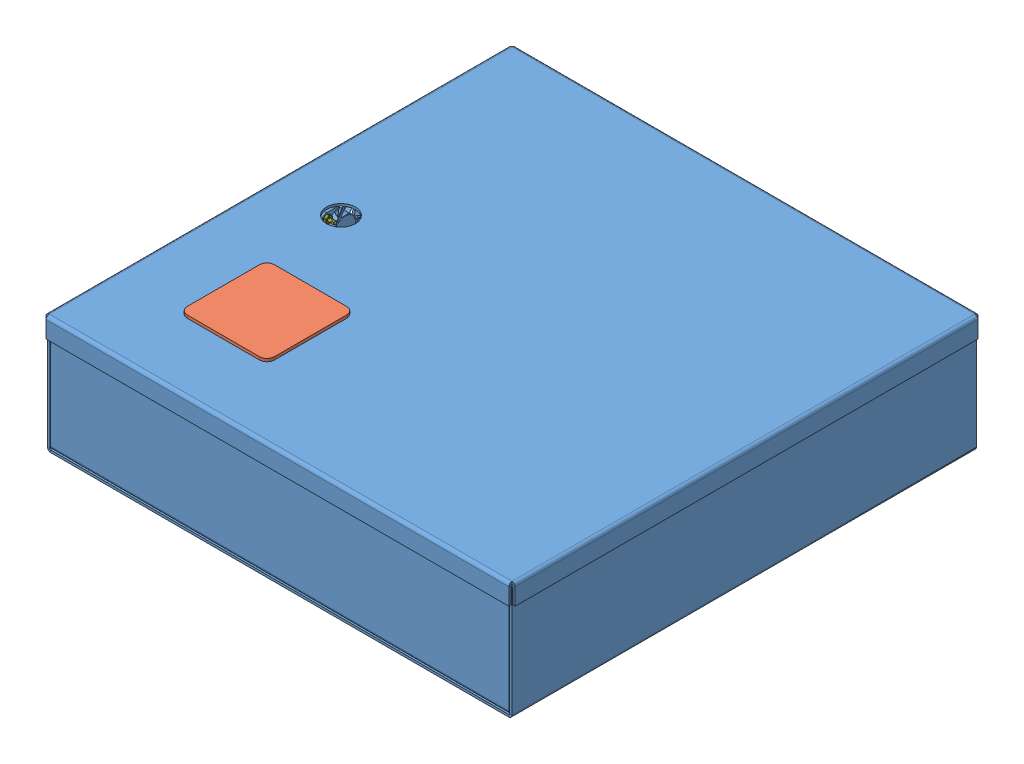
SolidWorks assembly elc box assebly, configuration Default. Lengths in mm.
Overall size (410.46 136 412.7).
107 component instances, 22 part files, 29 mates.
Components (placement in the parent):
- Electrical Enclosure 16 in-1: Electrical Enclosure 16 in [Default] at (-5.7869 193.9093 67.1276) size (410.46 103.63 410.46)
- elc component panel-1: elc component panel [Default] at (423.6423 -1.464 537.2069) x (-1 0 0) z (0 0 -1) size (400.05 136 400.05)
  - elc plate-1: elc plate [Default] at (226.2293 207.4053 266.8793) size (400.05 1.59 400.05)
  - power supply with standoffs-1: power supply with standoffs [Default] at (-1.4024 133.9192 27.3055) size (115.2 58.27 215)
    - __-1: __ [По умолчанию] at (110.1067 83.0736 152.0488) size (115.2 50.11 215)
    - 95783A055_NYLON 6 6 MALE-FEMALE THREADED HEX STANDOFF-1: 95783A055_NYLON 6 6 MALE-FEMALE THREADED HEX STANDOFF [95783A055] at (85.1067 81.4236 77.0488) x (0 1 0) z (0 0 1) size (13.03 5.2 4.5)
    - 95783A055_NYLON 6 6 MALE-FEMALE THREADED HEX STANDOFF-2: 95783A055_NYLON 6 6 MALE-FEMALE THREADED HEX STANDOFF [95783A055] at (135.1067 81.4236 77.0488) x (0 1 0) z (-0.939028 0 -0.343839) size (13.03 5.2 4.5)
    - 95783A055_NYLON 6 6 MALE-FEMALE THREADED HEX STANDOFF-3: 95783A055_NYLON 6 6 MALE-FEMALE THREADED HEX STANDOFF [95783A055] at (135.1067 81.4236 227.0488) x (0 1 0) z (-0.996262 0 -0.086381) size (13.03 5.2 4.5)
    - 95783A055_NYLON 6 6 MALE-FEMALE THREADED HEX STANDOFF-4: 95783A055_NYLON 6 6 MALE-FEMALE THREADED HEX STANDOFF [95783A055] at (85.1067 81.4236 227.0488) x (0 1 0) z (-0.990494 0 -0.137554) size (13.03 5.2 4.5)
  - arduino board assembly-1: arduino board assembly [Default] at (144.0018 173.6976 442.1285) x (0 0 -1) z (1 0 0) size (100 30.86 52.88)
    - ArduinoMega2560 CORRECTED-1: ArduinoMega2560 CORRECTED [Default] at (48.9673 43.2952 72.715) size (100 11.65 51.63)
    - breakout board-1: breakout board [Default] at (48.9673 54.2952 72.715) size (100 7 51.63)
    - 95783A055_NYLON 6 6 MALE-FEMALE THREADED HEX STANDOFF-1: 95783A055_NYLON 6 6 MALE-FEMALE THREADED HEX STANDOFF [95783A055] at (84.2031 36.9452 49.5995) x (0 -1 0) z (0 0 1) size (13.03 5.2 4.5)
    - 95783A055_NYLON 6 6 MALE-FEMALE THREADED HEX STANDOFF-2: 95783A055_NYLON 6 6 MALE-FEMALE THREADED HEX STANDOFF [95783A055] at (3.483 36.9452 49.7272) x (0 -1 0) z (0 0 1) size (13.03 5.2 4.5)
    - 95783A055_NYLON 6 6 MALE-FEMALE THREADED HEX STANDOFF-3: 95783A055_NYLON 6 6 MALE-FEMALE THREADED HEX STANDOFF [95783A055] at (9.6911 36.9452 96.9805) x (0 -1 0) z (0 0 1) size (13.03 5.2 4.5)
    - 91290A110_BLACK-OXIDE CLASS 12.9 SOCKET HEAD CAP SCREW-1: 91290A110_BLACK-OXIDE CLASS 12.9 SOCKET HEAD CAP SCREW [91290A110] at (9.6911 39.2952 96.9805) x (1 0 0) z (0 -1 0) size (5.5 5.5 8.18)
    - 91290A110_BLACK-OXIDE CLASS 12.9 SOCKET HEAD CAP SCREW-2: 91290A110_BLACK-OXIDE CLASS 12.9 SOCKET HEAD CAP SCREW [91290A110] at (84.2031 39.2952 49.5995) x (1 0 0) z (0 -1 0) size (5.5 5.5 8.18)
    - 91290A110_BLACK-OXIDE CLASS 12.9 SOCKET HEAD CAP SCREW-3: 91290A110_BLACK-OXIDE CLASS 12.9 SOCKET HEAD CAP SCREW [91290A110] at (3.483 39.2952 49.7272) x (1 0 0) z (0 -1 0) size (5.5 5.5 8.18)
  - din rail assmbly-1: din rail assmbly [Default] at (168.8197 101.8607 336.151) x (0 0 -1) z (1 0 0) size (90.31 80.69 125)
    - DIN 59_0-1: DIN 59_0 [00] at (103.6081 107.1321 54.2926) size (35 7.5 125)
    - 3812830-1: 3812830 [Default] at (104.4524 140.3713 142.3959) x (0 0 1) z (-1 0 0) size (6.2 76.69 90.31)
      - 3812830A-1: 3812830A [Default] at (-75.9936 -29.2392 18.3443) size (6.2 76.69 90.31)
      - 3812830B-1: 3812830B [Default] at (-75.3936 25.9608 19.6) size (5 19.3 28)
    - 3812830-2: 3812830 [Default] at (104.4524 140.3713 148.5959) x (0 0 1) z (-1 0 0) size (6.2 76.69 90.31)
      - 3812830A-1: 3812830A [Default] at (-75.9936 -29.2392 18.3443) size (6.2 76.69 90.31)
      - 3812830B-1: 3812830B [Default] at (-75.3936 25.9608 19.6) size (5 19.3 28)
    - 3812830-3: 3812830 [Default] at (104.4524 140.3713 154.7959) x (0 0 1) z (-1 0 0) size (6.2 76.69 90.31)
      - 3812830A-1: 3812830A [Default] at (-75.9936 -29.2392 18.3443) size (6.2 76.69 90.31)
      - 3812830B-1: 3812830B [Default] at (-75.3936 25.9608 19.6) size (5 19.3 28)
    - 3812830-4: 3812830 [Default] at (104.4524 140.3713 160.9959) x (0 0 1) z (-1 0 0) size (6.2 76.69 90.31)
      - 3812830A-1: 3812830A [Default] at (-75.9936 -29.2392 18.3443) size (6.2 76.69 90.31)
      - 3812830B-1: 3812830B [Default] at (-75.3936 25.9608 19.6) size (5 19.3 28)
    - SEIMENS 8WA1 808 DIN RAIL END RETAINER-1: SEIMENS 8WA1 808 DIN RAIL END RETAINER [Default] at (102.6081 107.6321 61.4023) size (45 44.95 10)
    - dinrail_Terminal-1: dinrail_Terminal [Default] at (121.1081 114.6321 91.2023) size (48 46.85 5.15)
    - dinrail_Terminal-2: dinrail_Terminal [Default] at (121.1081 114.6321 96.3523) size (48 46.85 5.15)
    - dinrail_Terminal-3: dinrail_Terminal [Default] at (121.1081 114.6321 101.5023) size (48 46.85 5.15)
    - dinrail_Terminal-4: dinrail_Terminal [Default] at (121.1081 114.6321 106.6523) size (48 46.85 5.15)
    - dinrail_Terminal-5: dinrail_Terminal [Default] at (121.1081 114.6321 111.8023) size (48 46.85 5.15)
    - 3812830-5: 3812830 [Default] at (104.4524 140.3713 205.3459) x (0 0 1) z (-1 0 0) size (6.2 76.69 90.31)
      - 3812830A-1: 3812830A [Default] at (-75.9936 -29.2392 18.3443) size (6.2 76.69 90.31)
      - 3812830B-1: 3812830B [Default] at (-75.3936 25.9608 19.6) size (5 19.3 28)
    - 3812830-6: 3812830 [Default] at (104.4524 140.3713 199.1459) x (0 0 1) z (-1 0 0) size (6.2 76.69 90.31)
      - 3812830A-1: 3812830A [Default] at (-75.9936 -29.2392 18.3443) size (6.2 76.69 90.31)
      - 3812830B-1: 3812830B [Default] at (-75.3936 25.9608 19.6) size (5 19.3 28)
    - 3812830-7: 3812830 [Default] at (104.4524 140.3713 192.9459) x (0 0 1) z (-1 0 0) size (6.2 76.69 90.31)
      - 3812830A-1: 3812830A [Default] at (-75.9936 -29.2392 18.3443) size (6.2 76.69 90.31)
      - 3812830B-1: 3812830B [Default] at (-75.3936 25.9608 19.6) size (5 19.3 28)
    - dinrail_Terminal-6: dinrail_Terminal [Default] at (121.1081 114.6321 135.5523) size (48 46.85 5.15)
    - dinrail_Terminal-7: dinrail_Terminal [Default] at (121.1081 114.6321 140.7023) size (48 46.85 5.15)
    - dinrail_Terminal-8: dinrail_Terminal [Default] at (121.1081 114.6321 145.8523) size (48 46.85 5.15)
    - dinrail_Terminal-9: dinrail_Terminal [Default] at (121.1081 114.6321 151.0023) size (48 46.85 5.15)
    - dinrail_Terminal-10: dinrail_Terminal [Default] at (121.1081 114.6321 156.1523) size (48 46.85 5.15)
    - SEIMENS 8WA1 808 DIN RAIL END RETAINER-3: SEIMENS 8WA1 808 DIN RAIL END RETAINER [Default] at (102.6081 107.6321 166.3023) size (45 44.95 10)
  - arduino board assembly-2: arduino board assembly [Default] at (46.0623 173.6976 442.1285) x (0 0 -1) z (1 0 0) size (100 30.86 52.88)
    - ArduinoMega2560 CORRECTED-1: ArduinoMega2560 CORRECTED [Default] at (48.9673 43.2952 72.715) size (100 11.65 51.63)
    - breakout board-1: breakout board [Default] at (48.9673 54.2952 72.715) size (100 7 51.63)
    - 95783A055_NYLON 6 6 MALE-FEMALE THREADED HEX STANDOFF-1: 95783A055_NYLON 6 6 MALE-FEMALE THREADED HEX STANDOFF [95783A055] at (84.2031 36.9452 49.5995) x (0 -1 0) z (0 0 1) size (13.03 5.2 4.5)
    - 95783A055_NYLON 6 6 MALE-FEMALE THREADED HEX STANDOFF-2: 95783A055_NYLON 6 6 MALE-FEMALE THREADED HEX STANDOFF [95783A055] at (3.483 36.9452 49.7272) x (0 -1 0) z (0 0 1) size (13.03 5.2 4.5)
    - 95783A055_NYLON 6 6 MALE-FEMALE THREADED HEX STANDOFF-3: 95783A055_NYLON 6 6 MALE-FEMALE THREADED HEX STANDOFF [95783A055] at (9.6911 36.9452 96.9805) x (0 -1 0) z (0 0 1) size (13.03 5.2 4.5)
    - 91290A110_BLACK-OXIDE CLASS 12.9 SOCKET HEAD CAP SCREW-1: 91290A110_BLACK-OXIDE CLASS 12.9 SOCKET HEAD CAP SCREW [91290A110] at (9.6911 39.2952 96.9805) x (1 0 0) z (0 -1 0) size (5.5 5.5 8.18)
    - 91290A110_BLACK-OXIDE CLASS 12.9 SOCKET HEAD CAP SCREW-2: 91290A110_BLACK-OXIDE CLASS 12.9 SOCKET HEAD CAP SCREW [91290A110] at (84.2031 39.2952 49.5995) x (1 0 0) z (0 -1 0) size (5.5 5.5 8.18)
    - 91290A110_BLACK-OXIDE CLASS 12.9 SOCKET HEAD CAP SCREW-3: 91290A110_BLACK-OXIDE CLASS 12.9 SOCKET HEAD CAP SCREW [91290A110] at (3.483 39.2952 49.7272) x (1 0 0) z (0 -1 0) size (5.5 5.5 8.18)
  - small panduit 1-1: small panduit 1 [Default] at (435.7793 210.2628 310.0077) size (368.3 30.38 16.31)
  - small panduit 2-1: small panduit 2 [Default] at (196.2827 210.2628 -91.8457) x (0 0 -1) z (1 0 0) size (133.35 30.38 16.31)
  - small panduit 3-1: small panduit 3 [Default] at (581.8293 210.2628 160.3509) size (222.25 30.38 16.31)
  - small panduit 2-2: small panduit 2 [Default] at (70.2327 210.2628 57.8111) x (0 0 -1) z (1 0 0) size (133.35 30.38 16.31)
  - small panduit 2-3: small panduit 2 [Default] at (168.1721 210.2628 57.8111) x (0 0 -1) z (1 0 0) size (133.35 30.38 16.31)
  - small panduit 2-4: small panduit 2 [Default] at (266.1116 210.2628 57.8111) x (0 0 -1) z (1 0 0) size (133.35 30.38 16.31)
  - small panduit 2-5: small panduit 2 [Default] at (667.965 210.2628 443.3577) size (133.35 30.38 16.31)
  - 92497A200_ZINC YELLOW-CHROMATE PLATED STEEL HEX NUT-1: 92497A200_ZINC YELLOW-CHROMATE PLATED STEEL HEX NUT [92497A200] at (95.7896 206.2053 438.6455) x (1 0 0) z (0 1 0) size (5.5 6.35 2.78)
  - 92497A200_ZINC YELLOW-CHROMATE PLATED STEEL HEX NUT-2: 92497A200_ZINC YELLOW-CHROMATE PLATED STEEL HEX NUT [92497A200] at (95.6618 206.2053 357.9254) x (1 0 0) z (0 1 0) size (5.5 6.35 2.78)
  - 92497A200_ZINC YELLOW-CHROMATE PLATED STEEL HEX NUT-3: 92497A200_ZINC YELLOW-CHROMATE PLATED STEEL HEX NUT [92497A200] at (143.0428 206.2053 432.4374) x (1 0 0) z (0 1 0) size (5.5 6.35 2.78)
  - 92497A200_ZINC YELLOW-CHROMATE PLATED STEEL HEX NUT-4: 92497A200_ZINC YELLOW-CHROMATE PLATED STEEL HEX NUT [92497A200] at (193.729 206.2053 438.6455) x (1 0 0) z (0 1 0) size (5.5 6.35 2.78)
  - 92497A200_ZINC YELLOW-CHROMATE PLATED STEEL HEX NUT-5: 92497A200_ZINC YELLOW-CHROMATE PLATED STEEL HEX NUT [92497A200] at (193.6013 206.2053 357.9254) x (1 0 0) z (0 1 0) size (5.5 6.35 2.78)
  - 92497A200_ZINC YELLOW-CHROMATE PLATED STEEL HEX NUT-6: 92497A200_ZINC YELLOW-CHROMATE PLATED STEEL HEX NUT [92497A200] at (240.9823 206.2053 432.4374) x (1 0 0) z (0 1 0) size (5.5 6.35 2.78)
  - 92095A177_18-8 SS BUTTON-HEAD SOCKET CAP SCREW-1: 92095A177_18-8 SS BUTTON-HEAD SOCKET CAP SCREW [92095A177] at (133.7043 205.7553 254.3543) x (1 0 0) z (0 -1 0) size (5.7 5.7 6.94)
  - 92095A177_18-8 SS BUTTON-HEAD SOCKET CAP SCREW-2: 92095A177_18-8 SS BUTTON-HEAD SOCKET CAP SCREW [92095A177] at (83.7043 205.7553 254.3543) x (1 0 0) z (0 -1 0) size (5.7 5.7 6.94)
  - 92095A177_18-8 SS BUTTON-HEAD SOCKET CAP SCREW-3: 92095A177_18-8 SS BUTTON-HEAD SOCKET CAP SCREW [92095A177] at (133.7043 205.7553 104.3543) x (1 0 0) z (0 -1 0) size (5.7 5.7 6.94)
  - 92095A177_18-8 SS BUTTON-HEAD SOCKET CAP SCREW-4: 92095A177_18-8 SS BUTTON-HEAD SOCKET CAP SCREW [92095A177] at (83.7043 205.7553 104.3543) x (1 0 0) z (0 -1 0) size (5.7 5.7 6.94)
  - 94060A146_PAN HEAD DRILLING SCREW FOR METAL-1: 94060A146_PAN HEAD DRILLING SCREW FOR METAL [94060A146] at (70.2327 204.3097 431.8261) x (1 0 0) z (0 1 0) size (6.86 6.86 33.5)
  - 94060A146_PAN HEAD DRILLING SCREW FOR METAL-2: 94060A146_PAN HEAD DRILLING SCREW FOR METAL [94060A146] at (70.2327 204.3097 327.6861) x (1 0 0) z (0 1 0) size (6.86 6.86 33.5)
  - 94060A146_PAN HEAD DRILLING SCREW FOR METAL-3: 94060A146_PAN HEAD DRILLING SCREW FOR METAL [94060A146] at (168.1721 204.3097 327.6861) x (1 0 0) z (0 1 0) size (6.86 6.86 33.5)
  - 94060A146_PAN HEAD DRILLING SCREW FOR METAL-4: 94060A146_PAN HEAD DRILLING SCREW FOR METAL [94060A146] at (168.1721 204.3097 431.8261) x (1 0 0) z (0 1 0) size (6.86 6.86 33.5)
  - 94060A146_PAN HEAD DRILLING SCREW FOR METAL-5: 94060A146_PAN HEAD DRILLING SCREW FOR METAL [94060A146] at (266.1116 204.3097 431.8261) x (1 0 0) z (0 1 0) size (6.86 6.86 33.5)
  - 94060A146_PAN HEAD DRILLING SCREW FOR METAL-6: 94060A146_PAN HEAD DRILLING SCREW FOR METAL [94060A146] at (266.1116 204.3097 327.6861) x (1 0 0) z (0 1 0) size (6.86 6.86 33.5)
  - 94060A146_PAN HEAD DRILLING SCREW FOR METAL-7: 94060A146_PAN HEAD DRILLING SCREW FOR METAL [94060A146] at (293.95 204.3097 443.3577) x (1 0 0) z (0 1 0) size (6.86 6.86 33.5)
  - 94060A146_PAN HEAD DRILLING SCREW FOR METAL-8: 94060A146_PAN HEAD DRILLING SCREW FOR METAL [94060A146] at (398.09 204.3097 443.3577) x (1 0 0) z (0 1 0) size (6.86 6.86 33.5)
  - 94060A146_PAN HEAD DRILLING SCREW FOR METAL-9: 94060A146_PAN HEAD DRILLING SCREW FOR METAL [94060A146] at (386.2493 204.3097 160.3509) x (1 0 0) z (0 1 0) size (6.86 6.86 33.5)
  - 94060A146_PAN HEAD DRILLING SCREW FOR METAL-10: 94060A146_PAN HEAD DRILLING SCREW FOR METAL [94060A146] at (196.2827 204.3097 178.0293) x (1 0 0) z (0 1 0) size (6.86 6.86 33.5)
  - 94060A146_PAN HEAD DRILLING SCREW FOR METAL-11: 94060A146_PAN HEAD DRILLING SCREW FOR METAL [94060A146] at (196.2827 204.3097 282.1693) x (1 0 0) z (0 1 0) size (6.86 6.86 33.5)
  - 94060A146_PAN HEAD DRILLING SCREW FOR METAL-12: 94060A146_PAN HEAD DRILLING SCREW FOR METAL [94060A146] at (207.8143 204.3097 160.3509) x (1 0 0) z (0 1 0) size (6.86 6.86 33.5)
  - 94060A146_PAN HEAD DRILLING SCREW FOR METAL-13: 94060A146_PAN HEAD DRILLING SCREW FOR METAL [94060A146] at (388.7893 204.3097 310.0077) x (1 0 0) z (0 1 0) size (6.86 6.86 33.5)
  - 94060A146_PAN HEAD DRILLING SCREW FOR METAL-14: 94060A146_PAN HEAD DRILLING SCREW FOR METAL [94060A146] at (61.7643 204.3097 310.0077) x (1 0 0) z (0 1 0) size (6.86 6.86 33.5)
  - 94060A146_PAN HEAD DRILLING SCREW FOR METAL-15: 94060A146_PAN HEAD DRILLING SCREW FOR METAL [94060A146] at (233.1123 204.0397 232.5429) x (1 0 0) z (0 1 0) size (6.86 6.86 33.5)
  - 94060A146_PAN HEAD DRILLING SCREW FOR METAL-16: 94060A146_PAN HEAD DRILLING SCREW FOR METAL [94060A146] at (341.1123 204.0397 232.5429) x (1 0 0) z (0 1 0) size (6.86 6.86 33.5)
- 40x40x10 DC Fan-1: 40x40x10 DC Fan [Default] at (249.8006 244.7093 74.4096) size (49.86 40.69 10.5)
- 40x40x10 DC Fan-2: 40x40x10 DC Fan [Default] at (1.4951 244.7093 225.8776) x (0 0 -1) z (1 0 0) size (49.86 40.69 10.5)
- fan hole cover-1: fan hole cover [Default] at (90.1997 300.0813 377.5156) x (-1 0 0) z (0 0 1) size (76.2 12.7 76.2)
- 92095A185_18-8 SS BUTTON-HEAD SOCKET CAP SCREW-1: 92095A185_18-8 SS BUTTON-HEAD SOCKET CAP SCREW [92095A185] at (265.8026 260.7113 65.4776) x (-0.923728 -0.383049 0) z (0 0 -1) size (5.7 5.7 22.02)
- 92095A185_18-8 SS BUTTON-HEAD SOCKET CAP SCREW-2: 92095A185_18-8 SS BUTTON-HEAD SOCKET CAP SCREW [92095A185] at (233.7986 228.7073 65.4776) x (-0.923728 -0.383049 0) z (0 0 -1) size (5.7 5.7 22.02)
- 92095A185_18-8 SS BUTTON-HEAD SOCKET CAP SCREW-3: 92095A185_18-8 SS BUTTON-HEAD SOCKET CAP SCREW [92095A185] at (-7.4369 260.7113 241.8796) x (0 0 1) z (-1 0 0) size (5.7 5.7 22.02)
- 92095A185_18-8 SS BUTTON-HEAD SOCKET CAP SCREW-4: 92095A185_18-8 SS BUTTON-HEAD SOCKET CAP SCREW [92095A185] at (-7.4369 228.7073 209.8756) x (0 0 1) z (-1 0 0) size (5.7 5.7 22.02)
- 92497A200_ZINC YELLOW-CHROMATE PLATED STEEL HEX NUT-1: 92497A200_ZINC YELLOW-CHROMATE PLATED STEEL HEX NUT [92497A200] at (265.8006 260.7093 80.8596) size (5.5 6.35 2.78)
- 92497A200_ZINC YELLOW-CHROMATE PLATED STEEL HEX NUT-2: 92497A200_ZINC YELLOW-CHROMATE PLATED STEEL HEX NUT [92497A200] at (233.8006 228.7093 80.8596) size (5.5 6.35 2.78)
- 92497A200_ZINC YELLOW-CHROMATE PLATED STEEL HEX NUT-3: 92497A200_ZINC YELLOW-CHROMATE PLATED STEEL HEX NUT [92497A200] at (7.9451 228.7093 209.8776) x (0 0 -1) z (1 0 0) size (5.5 6.35 2.78)
- 92497A200_ZINC YELLOW-CHROMATE PLATED STEEL HEX NUT-4: 92497A200_ZINC YELLOW-CHROMATE PLATED STEEL HEX NUT [92497A200] at (7.9451 260.7093 241.8776) x (0 0 -1) z (1 0 0) size (5.5 6.35 2.78)
- IEC320-C20-1: IEC320-C20 [Default] at (337.2782 245.1157 67.3026) size (31 24 28.57)
Mates (geometry in assembly coordinates):
- Concentric1: concentric anti-aligned: cylinder of Electrical Enclosure 16 in-1 through (381.5631 193.9093 435.4276) axis (0 -1 0) radius 2.5798; cylinder of elc component panel-1/elc plate-1 through (381.5631 205.9403 435.4276) axis (0 1 0) radius 2.665
- Concentric2: concentric anti-aligned: cylinder of Electrical Enclosure 16 in-1 through (13.2631 193.9093 435.4276) axis (0 -1 0) radius 2.5798; cylinder of elc component panel-1/elc plate-1 through (13.2631 205.9403 435.4276) axis (0 1 0) radius 2.665
- Distance1: distance = 10 mm anti-aligned: plane of elc component panel-1/elc plate-1 through (197.4131 205.9413 270.3276) normal (0 -1 0); plane of Electrical Enclosure 16 in-1 through (-5.7869 195.9413 473.5276) normal (0 1 0)
- Coincident2: coincident aligned: circle of Electrical Enclosure 16 in-1; plane of 40x40x10 DC Fan-1 through (233.8006 228.7093 69.1596) normal (0 0 -1)
- Concentric3: concentric aligned: cylinder of Electrical Enclosure 16 in-1 through (249.8006 244.7093 69.1596) axis (0 0 -1) radius 20.0025; cylinder of 40x40x10 DC Fan-1 through (249.8006 244.7093 79.6596) axis (0 0 -1) radius 19
- Coincident3: coincident anti-aligned: plane of Electrical Enclosure 16 in-1 through (-3.7549 193.9093 473.5276) normal (1 0 0); plane of 40x40x10 DC Fan-2 through (-3.7549 228.7093 241.8776) normal (-1 0 0)
- Concentric4: concentric aligned: cylinder of Electrical Enclosure 16 in-1 through (-3.7549 244.7093 225.8776) axis (-1 0 0) radius 20.0025; cylinder of 40x40x10 DC Fan-2 through (6.7451 244.7093 225.8776) axis (-1 0 0) radius 19
- Coincident4: coincident anti-aligned: plane of Electrical Enclosure 16 in-1 through (-5.7869 297.5413 67.1276) normal (0 1 0); plane of fan hole cover-1 through (90.1997 297.5413 377.5156) normal (0 -1 0)
- Concentric5: concentric aligned: cylinder of Electrical Enclosure 16 in-1 through (90.1997 295.5093 377.5156) axis (0 1 0) radius 31.75; cylinder of fan hole cover-1 through (90.1997 287.3813 377.5156) axis (0 1 0) radius 31.75
- Parallel1: parallel aligned: plane of Electrical Enclosure 16 in-1 through (-7.8189 193.9093 67.1276) normal (-1 0 0); plane of fan hole cover-1 through (52.0997 297.5413 415.6156) normal (-1 0 0)
- Coincident6: coincident anti-aligned: plane of Electrical Enclosure 16 in-1 through (-5.7869 193.9093 67.1276) normal (0 0 -1); plane of 92095A185_18-8 SS BUTTON-HEAD SOCKET CAP SCREW-2 through (234.8902 226.0746 67.1276) normal (0 0 1)
- Concentric6: concentric aligned: cylinder of Electrical Enclosure 16 in-1 through (233.7986 228.7073 69.1596) axis (0 0 -1) radius 1.5875; cylinder of 92095A185_18-8 SS BUTTON-HEAD SOCKET CAP SCREW-2 through (233.7986 228.7073 65.4776) axis (0 0 -1) radius 2.85
- Coincident7: coincident anti-aligned: plane of Electrical Enclosure 16 in-1 through (-5.7869 193.9093 67.1276) normal (0 0 -1); plane of 92095A185_18-8 SS BUTTON-HEAD SOCKET CAP SCREW-1 through (266.8942 258.0786 67.1276) normal (0 0 1)
- Concentric7: concentric aligned: cylinder of Electrical Enclosure 16 in-1 through (265.8026 260.7113 69.1596) axis (0 0 -1) radius 1.5875; cylinder of 92095A185_18-8 SS BUTTON-HEAD SOCKET CAP SCREW-1 through (265.8026 260.7113 65.4776) axis (0 0 -1) radius 2.85
- Coincident8: coincident anti-aligned: plane of Electrical Enclosure 16 in-1 through (-5.7869 193.9093 473.5276) normal (-1 0 0); plane of 92095A185_18-8 SS BUTTON-HEAD SOCKET CAP SCREW-4 through (-5.7869 225.8573 209.8756) normal (1 0 0)
- Coincident9: coincident anti-aligned: plane of Electrical Enclosure 16 in-1 through (-5.7869 193.9093 473.5276) normal (-1 0 0); plane of 92095A185_18-8 SS BUTTON-HEAD SOCKET CAP SCREW-3 through (-5.7869 257.8613 241.8796) normal (1 0 0)
- Concentric8: concentric aligned: cylinder of Electrical Enclosure 16 in-1 through (-3.7549 260.7113 241.8796) axis (-1 0 0) radius 1.5875; cylinder of 92095A185_18-8 SS BUTTON-HEAD SOCKET CAP SCREW-3 through (-7.4369 260.7113 241.8796) axis (-1 0 0) radius 2.85
- Concentric9: concentric aligned: cylinder of Electrical Enclosure 16 in-1 through (-3.7549 228.7073 209.8756) axis (-1 0 0) radius 1.5875; cylinder of 92095A185_18-8 SS BUTTON-HEAD SOCKET CAP SCREW-4 through (-7.4369 228.7073 209.8756) axis (-1 0 0) radius 2.85
- Coincident10: coincident anti-aligned: plane of 40x40x10 DC Fan-1 through (249.8006 244.7093 79.6596) normal (0 0 1); plane of 92497A200_ZINC YELLOW-CHROMATE PLATED STEEL HEX NUT-1 through (263.0506 262.297 79.6596) normal (0 0 -1)
- Concentric10: concentric aligned: cylinder of 40x40x10 DC Fan-1 through (265.8006 260.7093 79.6596) axis (0 0 1) radius 1.725; circle of 92497A200_ZINC YELLOW-CHROMATE PLATED STEEL HEX NUT-1
- Coincident11: coincident anti-aligned: plane of 40x40x10 DC Fan-1 through (249.8006 244.7093 79.6596) normal (0 0 1); plane of 92497A200_ZINC YELLOW-CHROMATE PLATED STEEL HEX NUT-2 through (231.0506 230.297 79.6596) normal (0 0 -1)
- Concentric11: concentric aligned: cylinder of 40x40x10 DC Fan-1 through (233.8006 228.7093 79.6596) axis (0 0 1) radius 1.725; circle of 92497A200_ZINC YELLOW-CHROMATE PLATED STEEL HEX NUT-2
- Coincident12: coincident anti-aligned: plane of 40x40x10 DC Fan-2 through (6.7451 244.7093 225.8776) normal (1 0 0); plane of 92497A200_ZINC YELLOW-CHROMATE PLATED STEEL HEX NUT-3 through (6.7451 230.297 212.6276) normal (-1 0 0)
- Concentric12: concentric aligned: cylinder of 40x40x10 DC Fan-2 through (6.7451 228.7093 209.8776) axis (1 0 0) radius 1.725; circle of 92497A200_ZINC YELLOW-CHROMATE PLATED STEEL HEX NUT-3
- Coincident13: coincident anti-aligned: plane of 40x40x10 DC Fan-2 through (6.7451 244.7093 225.8776) normal (1 0 0); plane of 92497A200_ZINC YELLOW-CHROMATE PLATED STEEL HEX NUT-4 through (6.7451 262.297 244.6276) normal (-1 0 0)
- Concentric13: concentric aligned: cylinder of 40x40x10 DC Fan-2 through (6.7451 260.7093 241.8776) axis (1 0 0) radius 1.725; circle of 92497A200_ZINC YELLOW-CHROMATE PLATED STEEL HEX NUT-4
- Coincident14: coincident anti-aligned: plane of Electrical Enclosure 16 in-1 through (-5.7869 193.9093 67.1276) normal (0 0 -1); plane of IEC320-C20-1 through (354.3282 231.5657 67.1276) normal (0 0 1)
- Coincident15: coincident anti-aligned: plane of Electrical Enclosure 16 in-1 through (350.6132 234.4604 473.5286) normal (-1 0 0); plane of IEC320-C20-1 through (350.6132 241.1986 67.1276) normal (1 0 0)
- Coincident16: coincident anti-aligned: plane of Electrical Enclosure 16 in-1 through (350.6132 254.9582 473.5286) normal (0 -1 0); plane of IEC320-C20-1 through (344.8982 254.9582 67.1276) normal (0 1 0)
